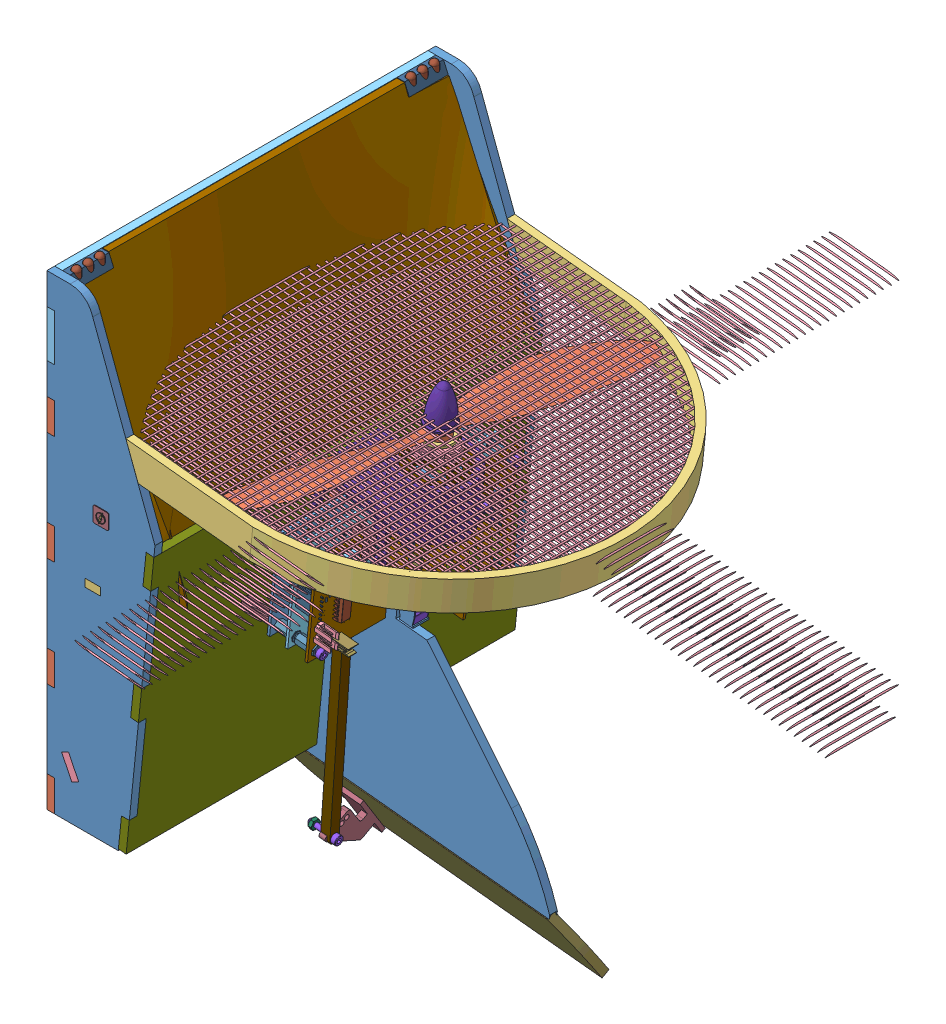
SolidWorks assembly AssTotaleSimu4, configuration Défaut. Lengths in mm.
Overall size (253.25 382.9 251.6).
1779 component instances, 238 part files, 11 mates.
Components (placement in the parent):
- AssStructSimu-1: AssStructSimu [Défaut] at (-125.7658 -1.8483 624.6548) x (1 0 0) z (0 0 -1) size (253.25 324.59 251.6)
  - AssBase-1: AssBase [Défaut] at (36.5482 -71.0398 34.0612) size (86.08 302.3 251.6)
    - AssD-1: AssD [Défaut] at (39.0992 31.0201 8.5) size (69.5 300 22)
      - P1-1: P1 [Défaut] at (-95.5819 194.6656 377.5) size (69.5 300 5)
      - P5-1: P5 [Défaut] at (-100.5819 -35.3344 360.5) x (0 1 0) z (1 0 0) size (230 22 5)
    - AssG-1: AssG [Défaut] at (39.0992 31.0201 -236.5) size (69.5 300 22)
      - P1-1: P1 [Défaut] at (-95.5819 194.6656 377.5) size (69.5 300 5)
      - P5-1: P5 [Défaut] at (-95.5819 -35.3344 399.5) x (0 1 0) z (-1 0 0) size (230 22 5)
    - P7-1: P7 [Défaut] at (-1.4828 89.6857 370.5) x (0 0 -1) z (0 -1 0) size (250 54.5 5)
    - P4-1: P4 [Défaut] at (-63.2363 165.9323 386) x (0 0 -1) z (0.898794 -0.438371 0) size (250 60.5 66.27)
    - P3-1: P3 [Défaut] at (-56.4828 -74.3143 146) x (0 0 1) z (-1 0 0) size (250 70 5)
    - P4b-1: P4b [Défaut] at (-58.7423 163.7404 190) x (0 0 1) z (0.438371 0.898794 0) size (152 56 2)
    - battery-1: battery [Défaut] at (-39.0156 204.1861 197.5) x (0 0 1) z (0.898794 -0.438371 0) size (137 43 30)
    - socket head cap screw 4762_din-1: socket head cap screw 4762_din [EN ISO 4762 M3 x 10 - 10N] at (-27.7008 145.2627 193) x (0.438371 0.898794 0) z (0 0 -1) size (13 5.5 5.5)
    - socket head cap screw 4762_din-2: socket head cap screw 4762_din [EN ISO 4762 M3 x 10 - 10N] at (-27.7008 145.2627 339) x (0.438371 0.898794 0) z (-0.791285 0.385936 -0.474259) size (13 5.5 5.5)
    - socket head cap screw 4762_din-3: socket head cap screw 4762_din [EN ISO 4762 M3 x 10 - 10N] at (-42.0815 152.2766 339) x (0.438371 0.898794 0) z (-0.001489 0.000726 -0.999999) size (13 5.5 5.5)
    - socket head cap screw 4762_din-4: socket head cap screw 4762_din [EN ISO 4762 M3 x 10 - 10N] at (-42.0815 152.2766 193) x (0.438371 0.898794 0) z (-0.031331 0.015281 -0.999392) size (13 5.5 5.5)
    - P11-1: P11 [Défaut] at (-57.5734 -73.9703 146.7843) x (0.005072 0 0.999987) z (0.006197 0.999981 -0.000031) size (240 65 164)
    - AssPhare-1: AssPhare [Défaut] at (-52.8518 -67.6977 411) x (0 1 0) z (0 0 -1) size (40.8 8 27.06)
      - piece_led-1: piece_led [Défaut] at (-6.6166 -3.631 25) size (7 8 25)
      - LED 5mm-1: LED 5mm [Valor predeterminado] at (-0.1166 0.369 30) x (0 0 1) z (-1 0 0) size (10.06 6 40.8)
      - LED 5mm-2: LED 5mm [Valor predeterminado] at (-0.1166 0.369 37.5) x (0 0 1) z (-1 0 0) size (10.06 6 40.8)
      - LED 5mm-3: LED 5mm [Valor predeterminado] at (-0.1166 0.369 45) x (0 0 1) z (-1 0 0) size (10.06 6 40.8)
    - AssPhare-2: AssPhare [Défaut] at (-52.8518 -67.6977 196) x (0 1 0) z (0 0 -1) size (40.8 8 27.06)
      - piece_led-1: piece_led [Défaut] at (-6.6166 -3.631 25) size (7 8 25)
      - LED 5mm-1: LED 5mm [Valor predeterminado] at (-0.1166 0.369 30) x (0 0 1) z (-1 0 0) size (10.06 6 40.8)
      - LED 5mm-2: LED 5mm [Valor predeterminado] at (-0.1166 0.369 37.5) x (0 0 1) z (-1 0 0) size (10.06 6 40.8)
      - LED 5mm-3: LED 5mm [Valor predeterminado] at (-0.1166 0.369 45) x (0 0 1) z (-1 0 0) size (10.06 6 40.8)
    - AssLogo-1: AssLogo [Défaut] at (-27.8835 45.1673 148.1054) x (-1 0 0) z (0 0 -1) size (10 10 0.8)
      - logo1-1: logo1 [Défaut] at (-6.5271 -4.4734 6.5054) size (5.8 7.71 0.4)
      - logo2-1: logo2 [Défaut] at (-6.4007 -4.4815 7.1054) size (10 10 0.4)
    - AssLogo-2: AssLogo [Défaut] at (-25.082 45.1673 383.8946) size (10 10 0.8)
      - logo1-1: logo1 [Défaut] at (-6.5271 -4.4734 6.5054) size (5.8 7.71 0.4)
      - logo2-1: logo2 [Défaut] at (-6.4007 -4.4815 7.1054) size (10 10 0.4)
    - support2-1: support2 [Défaut] at (-61.5648 191.7124 276) x (-0.017452 -0.999848 0) z (0.999848 -0.017452 0) size (75 20 10)
    - socket head cap screw 4762_din-5: socket head cap screw 4762_din [EN ISO 4762 M3 x 5 - 5N] at (-61.652 186.7132 269.3333) x (0.999848 -0.017452 0) z (-0.002158 -0.123615 0.992328) size (8 5.5 5.5)
    - socket head cap screw 4762_din-6: socket head cap screw 4762_din [EN ISO 4762 M3 x 5 - 5N] at (-61.652 186.7132 262.6667) x (0.999848 -0.017452 0) z (0 0 1) size (8 5.5 5.5)
    - socket head cap screw 4762_din-7: socket head cap screw 4762_din [EN ISO 4762 M3 x 25 - 18N] at (-55.2963 121.0922 253) x (0 0 1) z (-1 0 0) size (28 5.5 5.5)
    - hex nut style 1 gradeab_din-1: hex nut style 1 gradeab_din [Hexagon Nut ISO 4032 - M3 - W - N] at (-55.2963 121.0922 276) x (-0.923728 -0.383049 0) z (0 0 -1) size (5.5 6.35 2.4)
  - AssToitMot-1: AssToitMot [Défaut] at (-168.5238 43.6961 238.494) x (0 0 -1) z (0.9948 0.101852 0) size (250 207.5 205)
    - AssToit-1: AssToit [Défaut] at (-23.0702 -16.5789 -3.7148) size (250 207.5 205)
      - P8-1: P8 [Défaut] at (-38.4971 122.5921 203.5) size (250 175 5)
      - P12-1: P12 [Défaut] at (-60.4971 -63.4079 265.5) x (1 0 0) z (0 -1 0) size (44.28 76.64 55)
      - P13-1: P13 [Défaut] at (-35.9971 -52.8579 208.5) x (0 0 1) z (-1 0 0) size (64 15.55 5)
      - P10_2-1: P10_2 [Défaut] at (-35.9971 111.5921 171) x (0 0 1) z (-1 0 0) size (188.5 117.6 5)
    - Parallax-Servo_DUMMY-1: Parallax-Servo_DUMMY [Défaut] at (-61.6002 -51.5207 216.6662) x (1 0 0) z (0 1 0) size (20.07 42.67 55.64)
    - socket head cap screw 4762_din-1: socket head cap screw 4762_din [EN ISO 4762 M2.5 x 5 - 5N] at (-51.9272 -76.4868 259.2852) x (0 -1 0) z (-0.546944 0 0.837169) size (7.5 4.5 4.5)
    - socket head cap screw 4762_din-2: socket head cap screw 4762_din [EN ISO 4762 M2.5 x 5 - 5N] at (-61.5672 -76.4868 268.9252) x (0 -1 0) z (-0.546944 0 0.837169) size (7.5 4.5 4.5)
    - socket head cap screw 4762_din-3: socket head cap screw 4762_din [EN ISO 4762 M2.5 x 5 - 5N] at (-71.2072 -76.4868 259.2852) x (0 -1 0) z (-0.546944 0 0.837169) size (7.5 4.5 4.5)
    - socket head cap screw 4762_din-4: socket head cap screw 4762_din [EN ISO 4762 M2.5 x 5 - 5N] at (-61.5672 -76.4868 249.6452) x (0 -1 0) z (-0.546944 0 0.837169) size (7.5 4.5 4.5)
    - AssPhare-1: AssPhare [Défaut] at (8.4328 83.3966 196.1542) x (0 -1 0) z (1 0 0) size (40.8 8 27.06)
      - piece_led-1: piece_led [Défaut] at (-6.6166 -3.631 25) size (7 8 25)
      - LED 5mm-1: LED 5mm [Valor predeterminado] at (-0.1166 0.369 30) x (0 0 1) z (-1 0 0) size (10.06 6 40.8)
      - LED 5mm-2: LED 5mm [Valor predeterminado] at (-0.1166 0.369 37.5) x (0 0 1) z (-1 0 0) size (10.06 6 40.8)
      - LED 5mm-3: LED 5mm [Valor predeterminado] at (-0.1166 0.369 45) x (0 0 1) z (-1 0 0) size (10.06 6 40.8)
    - AssPhare-2: AssPhare [Défaut] at (-206.5672 83.3966 196.1542) x (0 -1 0) z (1 0 0) size (40.8 8 27.06)
      - piece_led-1: piece_led [Défaut] at (-6.6166 -3.631 25) size (7 8 25)
      - LED 5mm-1: LED 5mm [Valor predeterminado] at (-0.1166 0.369 30) x (0 0 1) z (-1 0 0) size (10.06 6 40.8)
      - LED 5mm-2: LED 5mm [Valor predeterminado] at (-0.1166 0.369 37.5) x (0 0 1) z (-1 0 0) size (10.06 6 40.8)
      - LED 5mm-3: LED 5mm [Valor predeterminado] at (-0.1166 0.369 45) x (0 0 1) z (-1 0 0) size (10.06 6 40.8)
    - socket head cap screw 4762_din-5: socket head cap screw 4762_din [EN ISO 4762 M3 x 10 - 10N] at (-67.0672 -22.9368 210.2852) x (0 0 -1) z (1 0 0) size (13 5.5 5.5)
    - socket head cap screw 4762_din-6: socket head cap screw 4762_din [EN ISO 4762 M3 x 10 - 10N] at (-56.0672 -72.9868 210.2852) x (0 0 -1) z (1 0 0) size (13 5.5 5.5)
    - socket head cap screw 4762_din-7: socket head cap screw 4762_din [EN ISO 4762 M3 x 10 - 10N] at (-67.0672 -72.9868 210.2852) x (0 0 -1) z (1 0 0) size (13 5.5 5.5)
    - socket head cap screw 4762_din-8: socket head cap screw 4762_din [EN ISO 4762 M3 x 10 - 10N] at (-56.0672 -22.9368 210.2852) x (0 0 -1) z (1 0 0) size (13 5.5 5.5)
    - hex nut style 1 gradeab_din-1: hex nut style 1 gradeab_din [Hexagon Nut ISO 4032 - M3 - W - N] at (-67.0672 -72.9868 197.3852) x (-0.923728 -0.383049 0) z (0 0 -1) size (5.5 6.35 2.4)
    - hex nut style 1 gradeab_din-2: hex nut style 1 gradeab_din [Hexagon Nut ISO 4032 - M3 - W - N] at (-56.0672 -72.9868 199.7852) size (5.5 6.35 2.4)
    - hex nut style 1 gradeab_din-3: hex nut style 1 gradeab_din [Hexagon Nut ISO 4032 - M3 - W - N] at (-67.0672 -22.9368 199.7852) size (5.5 6.35 2.4)
    - hex nut style 1 gradeab_din-4: hex nut style 1 gradeab_din [Hexagon Nut ISO 4032 - M3 - W - N] at (-56.0672 -22.9368 199.7852) size (5.5 6.35 2.4)
  - AssProtec-1: AssProtec [Défaut] at (86.6746 190.4649 284.6351) x (0 0 -1) z (0.101852 -0.9948 0) size (250 237.46 20)
    - protec3c-1: protec3c [Défaut] at (-140.4261 -87.7568 240) size (250 197 20)
    - AssGrillage-1: AssGrillage [Défaut] at (-370.4609 -132.5428 258.3161) x (0 0 -1) z (1 0 0) size (2.02 237.05 250)
      - barreau-1: barreau [Défaut] at (-1.1839 0.254 200) size (1 1 400)
      - barreau-3: barreau [Défaut] at (-1.1839 5.254 200) size (1 1 400)
      - barreau-4: barreau [Défaut] at (-1.1839 10.254 200) size (1 1 400)
      - barreau-5: barreau [Défaut] at (-1.1839 15.254 200) size (1 1 400)
      - barreau-6: barreau [Défaut] at (-1.1839 20.254 200) size (1 1 400)
      - barreau-7: barreau [Défaut] at (-1.1839 25.254 200) size (1 1 400)
      - barreau-8: barreau [Défaut] at (-1.1839 30.254 200) size (1 1 400)
      - barreau-9: barreau [Défaut] at (-1.1839 35.254 200) size (1 1 400)
      - barreau-10: barreau [Défaut] at (-1.1839 40.254 200) size (1 1 400)
      - barreau-11: barreau [Défaut] at (-1.1839 45.254 200) size (1 1 400)
      - barreau-12: barreau [Défaut] at (-1.1839 50.254 200) size (1 1 400)
      - barreau-13: barreau [Défaut] at (-1.1839 55.254 200) size (1 1 400)
      - barreau-14: barreau [Défaut] at (-1.1839 60.254 200) size (1 1 400)
      - barreau-15: barreau [Défaut] at (-1.1839 65.254 200) size (1 1 400)
      - barreau-16: barreau [Défaut] at (-1.1839 70.254 200) size (1 1 400)
      - barreau-17: barreau [Défaut] at (-1.1839 75.254 200) size (1 1 400)
      - barreau-18: barreau [Défaut] at (-1.1839 80.254 200) size (1 1 400)
      - barreau-19: barreau [Défaut] at (-1.1839 85.254 200) size (1 1 400)
      - barreau-20: barreau [Défaut] at (-1.1839 90.254 200) size (1 1 400)
      - barreau-21: barreau [Défaut] at (-1.1839 95.254 200) size (1 1 400)
      - barreau-22: barreau [Défaut] at (-1.1839 100.254 200) size (1 1 400)
      - barreau-23: barreau [Défaut] at (-1.1839 105.254 200) size (1 1 400)
      - barreau-24: barreau [Défaut] at (-1.1839 110.254 200) size (1 1 400)
      - barreau-25: barreau [Défaut] at (-1.1839 115.254 200) size (1 1 400)
      - barreau-26: barreau [Défaut] at (-1.1839 120.254 200) size (1 1 400)
      - barreau-27: barreau [Défaut] at (-1.1839 125.254 200) size (1 1 400)
      - barreau-28: barreau [Défaut] at (-1.1839 130.254 200) size (1 1 400)
      - barreau-29: barreau [Défaut] at (-1.1839 135.254 200) size (1 1 400)
      - barreau-30: barreau [Défaut] at (-1.1839 140.254 200) size (1 1 400)
      - barreau-31: barreau [Défaut] at (-1.1839 145.254 200) size (1 1 400)
      - barreau-32: barreau [Défaut] at (-1.1839 150.254 200) size (1 1 400)
      - barreau-33: barreau [Défaut] at (-1.1839 155.254 200) size (1 1 400)
      - barreau-34: barreau [Défaut] at (-1.1839 160.254 200) size (1 1 400)
      - barreau-35: barreau [Défaut] at (-1.1839 165.254 200) size (1 1 400)
      - barreau-36: barreau [Défaut] at (-1.1839 170.254 200) size (1 1 400)
      - barreau-37: barreau [Défaut] at (-1.1839 175.254 200) size (1 1 400)
      - barreau-38: barreau [Défaut] at (-1.1839 180.254 200) size (1 1 400)
      - barreau-39: barreau [Défaut] at (-1.1839 185.254 200) size (1 1 400)
      - barreau-40: barreau [Défaut] at (-1.1839 190.254 200) size (1 1 400)
      - barreau-41: barreau [Défaut] at (-1.1839 195.254 200) size (1 1 400)
      - barreau-42: barreau [Défaut] at (-0.1839 -1.5314 598.7823) x (0.998922 0 0.04641) z (0 1 0) size (1 1 400)
      - barreau-43: barreau [Défaut] at (-1.1839 200.254 200) size (1 1 400)
      - barreau-44: barreau [Défaut] at (-1.1839 205.254 200) size (1 1 400)
      - barreau-45: barreau [Défaut] at (-1.1839 210.254 200) size (1 1 400)
      - barreau-46: barreau [Défaut] at (-1.1839 215.254 200) size (1 1 400)
      - barreau-47: barreau [Défaut] at (-1.1839 220.254 200) size (1 1 400)
      - barreau-48: barreau [Défaut] at (-1.1839 225.254 200) size (1 1 400)
      - barreau-49: barreau [Défaut] at (-1.1839 230.254 200) size (1 1 400)
      - barreau-50: barreau [Défaut] at (-1.1839 235.254 200) size (1 1 400)
      - barreau-51: barreau [Défaut] at (-1.1839 240.254 200) size (1 1 400)
      - barreau-52: barreau [Défaut] at (-1.1839 245.254 200) size (1 1 400)
      - barreau-53: barreau [Défaut] at (-1.1839 250.254 200) size (1 1 400)
      - barreau-54: barreau [Défaut] at (-1.1839 255.254 200) size (1 1 400)
      - barreau-55: barreau [Défaut] at (-1.1839 260.254 200) size (1 1 400)
      - barreau-56: barreau [Défaut] at (-1.1839 265.254 200) size (1 1 400)
      - barreau-57: barreau [Défaut] at (-1.1839 270.254 200) size (1 1 400)
      - barreau-58: barreau [Défaut] at (-1.1839 275.254 200) size (1 1 400)
      - barreau-59: barreau [Défaut] at (-1.1839 280.254 200) size (1 1 400)
      - barreau-60: barreau [Défaut] at (-1.1839 285.254 200) size (1 1 400)
      - barreau-61: barreau [Défaut] at (-1.1839 290.254 200) size (1 1 400)
      - barreau-62: barreau [Défaut] at (-1.1839 295.254 200) size (1 1 400)
      - barreau-63: barreau [Défaut] at (-1.1839 300.254 200) size (1 1 400)
      - barreau-64: barreau [Défaut] at (-1.1839 305.254 200) size (1 1 400)
      - barreau-65: barreau [Défaut] at (-1.1839 310.254 200) size (1 1 400)
      - barreau-66: barreau [Défaut] at (-1.1839 315.254 200) size (1 1 400)
      - barreau-67: barreau [Défaut] at (-1.1839 320.254 200) size (1 1 400)
      - barreau-68: barreau [Défaut] at (-1.1839 325.254 200) size (1 1 400)
      - barreau-69: barreau [Défaut] at (-1.1839 330.254 200) size (1 1 400)
      - barreau-70: barreau [Défaut] at (-1.1839 335.254 200) size (1 1 400)
      - barreau-71: barreau [Défaut] at (-1.1839 340.254 200) size (1 1 400)
      - barreau-72: barreau [Défaut] at (-1.1839 345.254 200) size (1 1 400)
      - barreau-73: barreau [Défaut] at (-1.1839 350.254 200) size (1 1 400)
      - barreau-74: barreau [Défaut] at (-1.1839 355.254 200) size (1 1 400)
      - barreau-75: barreau [Défaut] at (-1.1839 360.254 200) size (1 1 400)
      - barreau-76: barreau [Défaut] at (-1.1839 365.254 200) size (1 1 400)
      - barreau-77: barreau [Défaut] at (-1.1839 370.254 200) size (1 1 400)
      - barreau-78: barreau [Défaut] at (-1.1839 375.254 200) size (1 1 400)
      - barreau-79: barreau [Défaut] at (-1.1839 380.254 200) size (1 1 400)
      - barreau-80: barreau [Défaut] at (-1.1839 385.254 200) size (1 1 400)
      - barreau-81: barreau [Défaut] at (-1.1839 390.254 200) size (1 1 400)
      - barreau-82: barreau [Défaut] at (-1.1839 395.254 200) size (1 1 400)
      - barreau-136: barreau [Défaut] at (-0.1839 -1.5314 593.7823) x (0.998922 0 0.04641) z (0 1 0) size (1 1 400)
      - barreau-137: barreau [Défaut] at (-0.1839 -1.5314 588.7823) x (0.998922 0 0.04641) z (0 1 0) size (1 1 400)
      - barreau-138: barreau [Défaut] at (-0.1839 -1.5314 583.7823) x (0.998922 0 0.04641) z (0 1 0) size (1 1 400)
      - barreau-139: barreau [Défaut] at (-0.1839 -1.5314 578.7823) x (0.998922 0 0.04641) z (0 1 0) size (1 1 400)
      - barreau-140: barreau [Défaut] at (-0.1839 -1.5314 573.7823) x (0.998922 0 0.04641) z (0 1 0) size (1 1 400)
      - barreau-141: barreau [Défaut] at (-0.1839 -1.5314 568.7823) x (0.998922 0 0.04641) z (0 1 0) size (1 1 400)
      - barreau-142: barreau [Défaut] at (-0.1839 -1.5314 563.7823) x (0.998922 0 0.04641) z (0 1 0) size (1 1 400)
      - barreau-143: barreau [Défaut] at (-0.1839 -1.5314 558.7823) x (0.998922 0 0.04641) z (0 1 0) size (1 1 400)
      - barreau-144: barreau [Défaut] at (-0.1839 -1.5314 553.7823) x (0.998922 0 0.04641) z (0 1 0) size (1 1 400)
      - barreau-145: barreau [Défaut] at (-0.1839 -1.5314 548.7823) x (0.998922 0 0.04641) z (0 1 0) size (1 1 400)
      - barreau-146: barreau [Défaut] at (-0.1839 -1.5314 543.7823) x (0.998922 0 0.04641) z (0 1 0) size (1 1 400)
      - barreau-147: barreau [Défaut] at (-0.1839 -1.5314 538.7823) x (0.998922 0 0.04641) z (0 1 0) size (1 1 400)
      - barreau-148: barreau [Défaut] at (-0.1839 -1.5314 533.7823) x (0.998922 0 0.04641) z (0 1 0) size (1 1 400)
      - barreau-149: barreau [Défaut] at (-0.1839 -1.5314 528.7823) x (0.998922 0 0.04641) z (0 1 0) size (1 1 400)
      - barreau-150: barreau [Défaut] at (-0.1839 -1.5314 523.7823) x (0.998922 0 0.04641) z (0 1 0) size (1 1 400)
      - barreau-151: barreau [Défaut] at (-0.1839 -1.5314 518.7823) x (0.998922 0 0.04641) z (0 1 0) size (1 1 400)
      - barreau-152: barreau [Défaut] at (-0.1839 -1.5314 513.7823) x (0.998922 0 0.04641) z (0 1 0) size (1 1 400)
      - barreau-153: barreau [Défaut] at (-0.1839 -1.5314 508.7823) x (0.998922 0 0.04641) z (0 1 0) size (1 1 400)
      - barreau-154: barreau [Défaut] at (-0.1839 -1.5314 503.7823) x (0.998922 0 0.04641) z (0 1 0) size (1 1 400)
      - barreau-155: barreau [Défaut] at (-0.1839 -1.5314 498.7823) x (0.998922 0 0.04641) z (0 1 0) size (1 1 400)
      - barreau-156: barreau [Défaut] at (-0.1839 -1.5314 493.7823) x (0.998922 0 0.04641) z (0 1 0) size (1 1 400)
      - barreau-157: barreau [Défaut] at (-0.1839 -1.5314 488.7823) x (0.998922 0 0.04641) z (0 1 0) size (1 1 400)
      - barreau-158: barreau [Défaut] at (-0.1839 -1.5314 483.7823) x (0.998922 0 0.04641) z (0 1 0) size (1 1 400)
      - barreau-159: barreau [Défaut] at (-0.1839 -1.5314 478.7823) x (0.998922 0 0.04641) z (0 1 0) size (1 1 400)
      - barreau-160: barreau [Défaut] at (-0.1839 -1.5314 473.7823) x (0.998922 0 0.04641) z (0 1 0) size (1 1 400)
      - barreau-161: barreau [Défaut] at (-0.1839 -1.5314 468.7823) x (0.998922 0 0.04641) z (0 1 0) size (1 1 400)
      - barreau-162: barreau [Défaut] at (-0.1839 -1.5314 463.7823) x (0.998922 0 0.04641) z (0 1 0) size (1 1 400)
      - barreau-163: barreau [Défaut] at (-0.1839 -1.5314 458.7823) x (0.998922 0 0.04641) z (0 1 0) size (1 1 400)
      - barreau-164: barreau [Défaut] at (-0.1839 -1.5314 453.7823) x (0.998922 0 0.04641) z (0 1 0) size (1 1 400)
      - barreau-165: barreau [Défaut] at (-0.1839 -1.5314 448.7823) x (0.998922 0 0.04641) z (0 1 0) size (1 1 400)
      - barreau-166: barreau [Défaut] at (-0.1839 -1.5314 443.7823) x (0.998922 0 0.04641) z (0 1 0) size (1 1 400)
      - barreau-167: barreau [Défaut] at (-0.1839 -1.5314 438.7823) x (0.998922 0 0.04641) z (0 1 0) size (1 1 400)
      - barreau-168: barreau [Défaut] at (-0.1839 -1.5314 433.7823) x (0.998922 0 0.04641) z (0 1 0) size (1 1 400)
      - barreau-169: barreau [Défaut] at (-0.1839 -1.5314 428.7823) x (0.998922 0 0.04641) z (0 1 0) size (1 1 400)
      - barreau-170: barreau [Défaut] at (-0.1839 -1.5314 423.7823) x (0.998922 0 0.04641) z (0 1 0) size (1 1 400)
      - barreau-171: barreau [Défaut] at (-0.1839 -1.5314 418.7823) x (0.998922 0 0.04641) z (0 1 0) size (1 1 400)
      - barreau-172: barreau [Défaut] at (-0.1839 -1.5314 413.7823) x (0.998922 0 0.04641) z (0 1 0) size (1 1 400)
      - barreau-173: barreau [Défaut] at (-0.1839 -1.5314 408.7823) x (0.998922 0 0.04641) z (0 1 0) size (1 1 400)
      - barreau-174: barreau [Défaut] at (-0.1839 -1.5314 403.7823) x (0.998922 0 0.04641) z (0 1 0) size (1 1 400)
      - barreau-175: barreau [Défaut] at (-0.1839 -1.5314 398.7823) x (0.998922 0 0.04641) z (0 1 0) size (1 1 400)
      - barreau-176: barreau [Défaut] at (-0.1839 -1.5314 393.7823) x (0.998922 0 0.04641) z (0 1 0) size (1 1 400)
      - barreau-177: barreau [Défaut] at (-0.1839 -1.5314 388.7823) x (0.998922 0 0.04641) z (0 1 0) size (1 1 400)
      - barreau-178: barreau [Défaut] at (-0.1839 -1.5314 383.7823) x (0.998922 0 0.04641) z (0 1 0) size (1 1 400)
      - barreau-179: barreau [Défaut] at (-0.1839 -1.5314 378.7823) x (0.998922 0 0.04641) z (0 1 0) size (1 1 400)
      - barreau-180: barreau [Défaut] at (-0.1839 -1.5314 373.7823) x (0.998922 0 0.04641) z (0 1 0) size (1 1 400)
      - barreau-181: barreau [Défaut] at (-0.1839 -1.5314 368.7823) x (0.998922 0 0.04641) z (0 1 0) size (1 1 400)
      - barreau-182: barreau [Défaut] at (-0.1839 -1.5314 363.7823) x (0.998922 0 0.04641) z (0 1 0) size (1 1 400)
      - barreau-183: barreau [Défaut] at (-0.1839 -1.5314 358.7823) x (0.998922 0 0.04641) z (0 1 0) size (1 1 400)
      - barreau-184: barreau [Défaut] at (-0.1839 -1.5314 353.7823) x (0.998922 0 0.04641) z (0 1 0) size (1 1 400)
      - barreau-185: barreau [Défaut] at (-0.1839 -1.5314 348.7823) x (0.998922 0 0.04641) z (0 1 0) size (1 1 400)
      - barreau-186: barreau [Défaut] at (-0.1839 -1.5314 343.7823) x (0.998922 0 0.04641) z (0 1 0) size (1 1 400)
      - barreau-187: barreau [Défaut] at (-0.1839 -1.5314 338.7823) x (0.998922 0 0.04641) z (0 1 0) size (1 1 400)
      - barreau-188: barreau [Défaut] at (-0.1839 -1.5314 333.7823) x (0.998922 0 0.04641) z (0 1 0) size (1 1 400)
      - barreau-189: barreau [Défaut] at (-0.1839 -1.5314 328.7823) x (0.998922 0 0.04641) z (0 1 0) size (1 1 400)
      - barreau-190: barreau [Défaut] at (-0.1839 -1.5314 323.7823) x (0.998922 0 0.04641) z (0 1 0) size (1 1 400)
      - barreau-191: barreau [Défaut] at (-0.1839 -1.5314 318.7823) x (0.998922 0 0.04641) z (0 1 0) size (1 1 400)
      - barreau-192: barreau [Défaut] at (-0.1839 -1.5314 313.7823) x (0.998922 0 0.04641) z (0 1 0) size (1 1 400)
      - barreau-193: barreau [Défaut] at (-0.1839 -1.5314 308.7823) x (0.998922 0 0.04641) z (0 1 0) size (1 1 400)
      - barreau-194: barreau [Défaut] at (-0.1839 -1.5314 303.7823) x (0.998922 0 0.04641) z (0 1 0) size (1 1 400)
      - barreau-195: barreau [Défaut] at (-0.1839 -1.5314 298.7823) x (0.998922 0 0.04641) z (0 1 0) size (1 1 400)
      - barreau-196: barreau [Défaut] at (-0.1839 -1.5314 293.7823) x (0.998922 0 0.04641) z (0 1 0) size (1 1 400)
      - barreau-197: barreau [Défaut] at (-0.1839 -1.5314 288.7823) x (0.998922 0 0.04641) z (0 1 0) size (1 1 400)
      - barreau-198: barreau [Défaut] at (-0.1839 -1.5314 283.7823) x (0.998922 0 0.04641) z (0 1 0) size (1 1 400)
      - barreau-199: barreau [Défaut] at (-0.1839 -1.5314 278.7823) x (0.998922 0 0.04641) z (0 1 0) size (1 1 400)
      - barreau-200: barreau [Défaut] at (-0.1839 -1.5314 273.7823) x (0.998922 0 0.04641) z (0 1 0) size (1 1 400)
      - barreau-201: barreau [Défaut] at (-0.1839 -1.5314 268.7823) x (0.998922 0 0.04641) z (0 1 0) size (1 1 400)
      - barreau-202: barreau [Défaut] at (-0.1839 -1.5314 263.7823) x (0.998922 0 0.04641) z (0 1 0) size (1 1 400)
      - barreau-203: barreau [Défaut] at (-0.1839 -1.5314 258.7823) x (0.998922 0 0.04641) z (0 1 0) size (1 1 400)
      - barreau-204: barreau [Défaut] at (-0.1839 -1.5314 253.7823) x (0.998922 0 0.04641) z (0 1 0) size (1 1 400)
      - barreau-205: barreau [Défaut] at (-0.1839 -1.5314 248.7823) x (0.998922 0 0.04641) z (0 1 0) size (1 1 400)
      - barreau-206: barreau [Défaut] at (-0.1839 -1.5314 243.7823) x (0.998922 0 0.04641) z (0 1 0) size (1 1 400)
      - barreau-207: barreau [Défaut] at (-0.1839 -1.5314 238.7823) x (0.998922 0 0.04641) z (0 1 0) size (1 1 400)
      - barreau-208: barreau [Défaut] at (-0.1839 -1.5314 233.7823) x (0.998922 0 0.04641) z (0 1 0) size (1 1 400)
      - barreau-209: barreau [Défaut] at (-0.1839 -1.5314 228.7823) x (0.998922 0 0.04641) z (0 1 0) size (1 1 400)
      - barreau-210: barreau [Défaut] at (-0.1839 -1.5314 223.7823) x (0.998922 0 0.04641) z (0 1 0) size (1 1 400)
      - barreau-211: barreau [Défaut] at (-0.1839 -1.5314 218.7823) x (0.998922 0 0.04641) z (0 1 0) size (1 1 400)
      - barreau-212: barreau [Défaut] at (-0.1839 -1.5314 213.7823) x (0.998922 0 0.04641) z (0 1 0) size (1 1 400)
      - barreau-213: barreau [Défaut] at (-0.1839 -1.5314 208.7823) x (0.998922 0 0.04641) z (0 1 0) size (1 1 400)
      - barreau-214: barreau [Défaut] at (-0.1839 -1.5314 203.7823) x (0.998922 0 0.04641) z (0 1 0) size (1 1 400)
    - AssGrillage-2: AssGrillage [Défaut] at (339.6086 -132.5428 241.6839) x (0 0 1) z (-1 0 0) size (2.02 237.05 250)
      - barreau-1: barreau [Défaut] at (-1.1839 0.254 200) size (1 1 400)
      - barreau-3: barreau [Défaut] at (-1.1839 5.254 200) size (1 1 400)
      - barreau-4: barreau [Défaut] at (-1.1839 10.254 200) size (1 1 400)
      - barreau-5: barreau [Défaut] at (-1.1839 15.254 200) size (1 1 400)
      - barreau-6: barreau [Défaut] at (-1.1839 20.254 200) size (1 1 400)
      - barreau-7: barreau [Défaut] at (-1.1839 25.254 200) size (1 1 400)
      - barreau-8: barreau [Défaut] at (-1.1839 30.254 200) size (1 1 400)
      - barreau-9: barreau [Défaut] at (-1.1839 35.254 200) size (1 1 400)
      - barreau-10: barreau [Défaut] at (-1.1839 40.254 200) size (1 1 400)
      - barreau-11: barreau [Défaut] at (-1.1839 45.254 200) size (1 1 400)
      - barreau-12: barreau [Défaut] at (-1.1839 50.254 200) size (1 1 400)
      - barreau-13: barreau [Défaut] at (-1.1839 55.254 200) size (1 1 400)
      - barreau-14: barreau [Défaut] at (-1.1839 60.254 200) size (1 1 400)
      - barreau-15: barreau [Défaut] at (-1.1839 65.254 200) size (1 1 400)
      - barreau-16: barreau [Défaut] at (-1.1839 70.254 200) size (1 1 400)
      - barreau-17: barreau [Défaut] at (-1.1839 75.254 200) size (1 1 400)
      - barreau-18: barreau [Défaut] at (-1.1839 80.254 200) size (1 1 400)
      - barreau-19: barreau [Défaut] at (-1.1839 85.254 200) size (1 1 400)
      - barreau-20: barreau [Défaut] at (-1.1839 90.254 200) size (1 1 400)
      - barreau-21: barreau [Défaut] at (-1.1839 95.254 200) size (1 1 400)
      - barreau-22: barreau [Défaut] at (-1.1839 100.254 200) size (1 1 400)
      - barreau-23: barreau [Défaut] at (-1.1839 105.254 200) size (1 1 400)
      - barreau-24: barreau [Défaut] at (-1.1839 110.254 200) size (1 1 400)
      - barreau-25: barreau [Défaut] at (-1.1839 115.254 200) size (1 1 400)
      - barreau-26: barreau [Défaut] at (-1.1839 120.254 200) size (1 1 400)
      - barreau-27: barreau [Défaut] at (-1.1839 125.254 200) size (1 1 400)
      - barreau-28: barreau [Défaut] at (-1.1839 130.254 200) size (1 1 400)
      - barreau-29: barreau [Défaut] at (-1.1839 135.254 200) size (1 1 400)
      - barreau-30: barreau [Défaut] at (-1.1839 140.254 200) size (1 1 400)
      - barreau-31: barreau [Défaut] at (-1.1839 145.254 200) size (1 1 400)
      - barreau-32: barreau [Défaut] at (-1.1839 150.254 200) size (1 1 400)
      - barreau-33: barreau [Défaut] at (-1.1839 155.254 200) size (1 1 400)
      - barreau-34: barreau [Défaut] at (-1.1839 160.254 200) size (1 1 400)
      - barreau-35: barreau [Défaut] at (-1.1839 165.254 200) size (1 1 400)
      - barreau-36: barreau [Défaut] at (-1.1839 170.254 200) size (1 1 400)
      - barreau-37: barreau [Défaut] at (-1.1839 175.254 200) size (1 1 400)
      - barreau-38: barreau [Défaut] at (-1.1839 180.254 200) size (1 1 400)
      - barreau-39: barreau [Défaut] at (-1.1839 185.254 200) size (1 1 400)
      - barreau-40: barreau [Défaut] at (-1.1839 190.254 200) size (1 1 400)
      - barreau-41: barreau [Défaut] at (-1.1839 195.254 200) size (1 1 400)
      - barreau-42: barreau [Défaut] at (-0.1839 -1.5314 598.7823) x (0.998922 0 0.04641) z (0 1 0) size (1 1 400)
      - barreau-43: barreau [Défaut] at (-1.1839 200.254 200) size (1 1 400)
      - barreau-44: barreau [Défaut] at (-1.1839 205.254 200) size (1 1 400)
      - barreau-45: barreau [Défaut] at (-1.1839 210.254 200) size (1 1 400)
      - barreau-46: barreau [Défaut] at (-1.1839 215.254 200) size (1 1 400)
      - barreau-47: barreau [Défaut] at (-1.1839 220.254 200) size (1 1 400)
      - barreau-48: barreau [Défaut] at (-1.1839 225.254 200) size (1 1 400)
      - barreau-49: barreau [Défaut] at (-1.1839 230.254 200) size (1 1 400)
      - barreau-50: barreau [Défaut] at (-1.1839 235.254 200) size (1 1 400)
      - barreau-51: barreau [Défaut] at (-1.1839 240.254 200) size (1 1 400)
      - barreau-52: barreau [Défaut] at (-1.1839 245.254 200) size (1 1 400)
      - barreau-53: barreau [Défaut] at (-1.1839 250.254 200) size (1 1 400)
      - barreau-54: barreau [Défaut] at (-1.1839 255.254 200) size (1 1 400)
      - barreau-55: barreau [Défaut] at (-1.1839 260.254 200) size (1 1 400)
      - barreau-56: barreau [Défaut] at (-1.1839 265.254 200) size (1 1 400)
      - barreau-57: barreau [Défaut] at (-1.1839 270.254 200) size (1 1 400)
      - barreau-58: barreau [Défaut] at (-1.1839 275.254 200) size (1 1 400)
      - barreau-59: barreau [Défaut] at (-1.1839 280.254 200) size (1 1 400)
      - barreau-60: barreau [Défaut] at (-1.1839 285.254 200) size (1 1 400)
      - barreau-61: barreau [Défaut] at (-1.1839 290.254 200) size (1 1 400)
      - barreau-62: barreau [Défaut] at (-1.1839 295.254 200) size (1 1 400)
      - barreau-63: barreau [Défaut] at (-1.1839 300.254 200) size (1 1 400)
      - barreau-64: barreau [Défaut] at (-1.1839 305.254 200) size (1 1 400)
      - barreau-65: barreau [Défaut] at (-1.1839 310.254 200) size (1 1 400)
      - barreau-66: barreau [Défaut] at (-1.1839 315.254 200) size (1 1 400)
      - barreau-67: barreau [Défaut] at (-1.1839 320.254 200) size (1 1 400)
      - barreau-68: barreau [Défaut] at (-1.1839 325.254 200) size (1 1 400)
      - barreau-69: barreau [Défaut] at (-1.1839 330.254 200) size (1 1 400)
      - barreau-70: barreau [Défaut] at (-1.1839 335.254 200) size (1 1 400)
      - barreau-71: barreau [Défaut] at (-1.1839 340.254 200) size (1 1 400)
      - barreau-72: barreau [Défaut] at (-1.1839 345.254 200) size (1 1 400)
      - barreau-73: barreau [Défaut] at (-1.1839 350.254 200) size (1 1 400)
      - barreau-74: barreau [Défaut] at (-1.1839 355.254 200) size (1 1 400)
      - barreau-75: barreau [Défaut] at (-1.1839 360.254 200) size (1 1 400)
      - barreau-76: barreau [Défaut] at (-1.1839 365.254 200) size (1 1 400)
      - barreau-77: barreau [Défaut] at (-1.1839 370.254 200) size (1 1 400)
      - barreau-78: barreau [Défaut] at (-1.1839 375.254 200) size (1 1 400)
      - barreau-79: barreau [Défaut] at (-1.1839 380.254 200) size (1 1 400)
      - barreau-80: barreau [Défaut] at (-1.1839 385.254 200) size (1 1 400)
      - barreau-81: barreau [Défaut] at (-1.1839 390.254 200) size (1 1 400)
      - barreau-82: barreau [Défaut] at (-1.1839 395.254 200) size (1 1 400)
      - barreau-136: barreau [Défaut] at (-0.1839 -1.5314 593.7823) x (0.998922 0 0.04641) z (0 1 0) size (1 1 400)
      - barreau-137: barreau [Défaut] at (-0.1839 -1.5314 588.7823) x (0.998922 0 0.04641) z (0 1 0) size (1 1 400)
      - barreau-138: barreau [Défaut] at (-0.1839 -1.5314 583.7823) x (0.998922 0 0.04641) z (0 1 0) size (1 1 400)
      - barreau-139: barreau [Défaut] at (-0.1839 -1.5314 578.7823) x (0.998922 0 0.04641) z (0 1 0) size (1 1 400)
      - barreau-140: barreau [Défaut] at (-0.1839 -1.5314 573.7823) x (0.998922 0 0.04641) z (0 1 0) size (1 1 400)
      - barreau-141: barreau [Défaut] at (-0.1839 -1.5314 568.7823) x (0.998922 0 0.04641) z (0 1 0) size (1 1 400)
      - barreau-142: barreau [Défaut] at (-0.1839 -1.5314 563.7823) x (0.998922 0 0.04641) z (0 1 0) size (1 1 400)
      - barreau-143: barreau [Défaut] at (-0.1839 -1.5314 558.7823) x (0.998922 0 0.04641) z (0 1 0) size (1 1 400)
      - barreau-144: barreau [Défaut] at (-0.1839 -1.5314 553.7823) x (0.998922 0 0.04641) z (0 1 0) size (1 1 400)
      - barreau-145: barreau [Défaut] at (-0.1839 -1.5314 548.7823) x (0.998922 0 0.04641) z (0 1 0) size (1 1 400)
      - barreau-146: barreau [Défaut] at (-0.1839 -1.5314 543.7823) x (0.998922 0 0.04641) z (0 1 0) size (1 1 400)
      - barreau-147: barreau [Défaut] at (-0.1839 -1.5314 538.7823) x (0.998922 0 0.04641) z (0 1 0) size (1 1 400)
      - barreau-148: barreau [Défaut] at (-0.1839 -1.5314 533.7823) x (0.998922 0 0.04641) z (0 1 0) size (1 1 400)
      - barreau-149: barreau [Défaut] at (-0.1839 -1.5314 528.7823) x (0.998922 0 0.04641) z (0 1 0) size (1 1 400)
      - barreau-150: barreau [Défaut] at (-0.1839 -1.5314 523.7823) x (0.998922 0 0.04641) z (0 1 0) size (1 1 400)
      - barreau-151: barreau [Défaut] at (-0.1839 -1.5314 518.7823) x (0.998922 0 0.04641) z (0 1 0) size (1 1 400)
      - barreau-152: barreau [Défaut] at (-0.1839 -1.5314 513.7823) x (0.998922 0 0.04641) z (0 1 0) size (1 1 400)
      - barreau-153: barreau [Défaut] at (-0.1839 -1.5314 508.7823) x (0.998922 0 0.04641) z (0 1 0) size (1 1 400)
      - barreau-154: barreau [Défaut] at (-0.1839 -1.5314 503.7823) x (0.998922 0 0.04641) z (0 1 0) size (1 1 400)
      - barreau-155: barreau [Défaut] at (-0.1839 -1.5314 498.7823) x (0.998922 0 0.04641) z (0 1 0) size (1 1 400)
      - barreau-156: barreau [Défaut] at (-0.1839 -1.5314 493.7823) x (0.998922 0 0.04641) z (0 1 0) size (1 1 400)
      - barreau-157: barreau [Défaut] at (-0.1839 -1.5314 488.7823) x (0.998922 0 0.04641) z (0 1 0) size (1 1 400)
      - barreau-158: barreau [Défaut] at (-0.1839 -1.5314 483.7823) x (0.998922 0 0.04641) z (0 1 0) size (1 1 400)
      - barreau-159: barreau [Défaut] at (-0.1839 -1.5314 478.7823) x (0.998922 0 0.04641) z (0 1 0) size (1 1 400)
      - barreau-160: barreau [Défaut] at (-0.1839 -1.5314 473.7823) x (0.998922 0 0.04641) z (0 1 0) size (1 1 400)
      - barreau-161: barreau [Défaut] at (-0.1839 -1.5314 468.7823) x (0.998922 0 0.04641) z (0 1 0) size (1 1 400)
      - barreau-162: barreau [Défaut] at (-0.1839 -1.5314 463.7823) x (0.998922 0 0.04641) z (0 1 0) size (1 1 400)
      - barreau-163: barreau [Défaut] at (-0.1839 -1.5314 458.7823) x (0.998922 0 0.04641) z (0 1 0) size (1 1 400)
      - barreau-164: barreau [Défaut] at (-0.1839 -1.5314 453.7823) x (0.998922 0 0.04641) z (0 1 0) size (1 1 400)
      - barreau-165: barreau [Défaut] at (-0.1839 -1.5314 448.7823) x (0.998922 0 0.04641) z (0 1 0) size (1 1 400)
      - barreau-166: barreau [Défaut] at (-0.1839 -1.5314 443.7823) x (0.998922 0 0.04641) z (0 1 0) size (1 1 400)
      - barreau-167: barreau [Défaut] at (-0.1839 -1.5314 438.7823) x (0.998922 0 0.04641) z (0 1 0) size (1 1 400)
      - barreau-168: barreau [Défaut] at (-0.1839 -1.5314 433.7823) x (0.998922 0 0.04641) z (0 1 0) size (1 1 400)
      - barreau-169: barreau [Défaut] at (-0.1839 -1.5314 428.7823) x (0.998922 0 0.04641) z (0 1 0) size (1 1 400)
      - barreau-170: barreau [Défaut] at (-0.1839 -1.5314 423.7823) x (0.998922 0 0.04641) z (0 1 0) size (1 1 400)
      - barreau-171: barreau [Défaut] at (-0.1839 -1.5314 418.7823) x (0.998922 0 0.04641) z (0 1 0) size (1 1 400)
      - barreau-172: barreau [Défaut] at (-0.1839 -1.5314 413.7823) x (0.998922 0 0.04641) z (0 1 0) size (1 1 400)
      - barreau-173: barreau [Défaut] at (-0.1839 -1.5314 408.7823) x (0.998922 0 0.04641) z (0 1 0) size (1 1 400)
      - barreau-174: barreau [Défaut] at (-0.1839 -1.5314 403.7823) x (0.998922 0 0.04641) z (0 1 0) size (1 1 400)
      - barreau-175: barreau [Défaut] at (-0.1839 -1.5314 398.7823) x (0.998922 0 0.04641) z (0 1 0) size (1 1 400)
      - barreau-176: barreau [Défaut] at (-0.1839 -1.5314 393.7823) x (0.998922 0 0.04641) z (0 1 0) size (1 1 400)
      - barreau-177: barreau [Défaut] at (-0.1839 -1.5314 388.7823) x (0.998922 0 0.04641) z (0 1 0) size (1 1 400)
      - barreau-178: barreau [Défaut] at (-0.1839 -1.5314 383.7823) x (0.998922 0 0.04641) z (0 1 0) size (1 1 400)
      - barreau-179: barreau [Défaut] at (-0.1839 -1.5314 378.7823) x (0.998922 0 0.04641) z (0 1 0) size (1 1 400)
      - barreau-180: barreau [Défaut] at (-0.1839 -1.5314 373.7823) x (0.998922 0 0.04641) z (0 1 0) size (1 1 400)
      - barreau-181: barreau [Défaut] at (-0.1839 -1.5314 368.7823) x (0.998922 0 0.04641) z (0 1 0) size (1 1 400)
      - barreau-182: barreau [Défaut] at (-0.1839 -1.5314 363.7823) x (0.998922 0 0.04641) z (0 1 0) size (1 1 400)
      - barreau-183: barreau [Défaut] at (-0.1839 -1.5314 358.7823) x (0.998922 0 0.04641) z (0 1 0) size (1 1 400)
      - barreau-184: barreau [Défaut] at (-0.1839 -1.5314 353.7823) x (0.998922 0 0.04641) z (0 1 0) size (1 1 400)
      - barreau-185: barreau [Défaut] at (-0.1839 -1.5314 348.7823) x (0.998922 0 0.04641) z (0 1 0) size (1 1 400)
      - barreau-186: barreau [Défaut] at (-0.1839 -1.5314 343.7823) x (0.998922 0 0.04641) z (0 1 0) size (1 1 400)
      - barreau-187: barreau [Défaut] at (-0.1839 -1.5314 338.7823) x (0.998922 0 0.04641) z (0 1 0) size (1 1 400)
      - barreau-188: barreau [Défaut] at (-0.1839 -1.5314 333.7823) x (0.998922 0 0.04641) z (0 1 0) size (1 1 400)
      - barreau-189: barreau [Défaut] at (-0.1839 -1.5314 328.7823) x (0.998922 0 0.04641) z (0 1 0) size (1 1 400)
      - barreau-190: barreau [Défaut] at (-0.1839 -1.5314 323.7823) x (0.998922 0 0.04641) z (0 1 0) size (1 1 400)
      - barreau-191: barreau [Défaut] at (-0.1839 -1.5314 318.7823) x (0.998922 0 0.04641) z (0 1 0) size (1 1 400)
      - barreau-192: barreau [Défaut] at (-0.1839 -1.5314 313.7823) x (0.998922 0 0.04641) z (0 1 0) size (1 1 400)
      - barreau-193: barreau [Défaut] at (-0.1839 -1.5314 308.7823) x (0.998922 0 0.04641) z (0 1 0) size (1 1 400)
      - barreau-194: barreau [Défaut] at (-0.1839 -1.5314 303.7823) x (0.998922 0 0.04641) z (0 1 0) size (1 1 400)
      - barreau-195: barreau [Défaut] at (-0.1839 -1.5314 298.7823) x (0.998922 0 0.04641) z (0 1 0) size (1 1 400)
      - barreau-196: barreau [Défaut] at (-0.1839 -1.5314 293.7823) x (0.998922 0 0.04641) z (0 1 0) size (1 1 400)
      - barreau-197: barreau [Défaut] at (-0.1839 -1.5314 288.7823) x (0.998922 0 0.04641) z (0 1 0) size (1 1 400)
      - barreau-198: barreau [Défaut] at (-0.1839 -1.5314 283.7823) x (0.998922 0 0.04641) z (0 1 0) size (1 1 400)
      - barreau-199: barreau [Défaut] at (-0.1839 -1.5314 278.7823) x (0.998922 0 0.04641) z (0 1 0) size (1 1 400)
      - barreau-200: barreau [Défaut] at (-0.1839 -1.5314 273.7823) x (0.998922 0 0.04641) z (0 1 0) size (1 1 400)
      - barreau-201: barreau [Défaut] at (-0.1839 -1.5314 268.7823) x (0.998922 0 0.04641) z (0 1 0) size (1 1 400)
      - barreau-202: barreau [Défaut] at (-0.1839 -1.5314 263.7823) x (0.998922 0 0.04641) z (0 1 0) size (1 1 400)
      - barreau-203: barreau [Défaut] at (-0.1839 -1.5314 258.7823) x (0.998922 0 0.04641) z (0 1 0) size (1 1 400)
      - barreau-204: barreau [Défaut] at (-0.1839 -1.5314 253.7823) x (0.998922 0 0.04641) z (0 1 0) size (1 1 400)
      - barreau-205: barreau [Défaut] at (-0.1839 -1.5314 248.7823) x (0.998922 0 0.04641) z (0 1 0) size (1 1 400)
      - barreau-206: barreau [Défaut] at (-0.1839 -1.5314 243.7823) x (0.998922 0 0.04641) z (0 1 0) size (1 1 400)
      - barreau-207: barreau [Défaut] at (-0.1839 -1.5314 238.7823) x (0.998922 0 0.04641) z (0 1 0) size (1 1 400)
